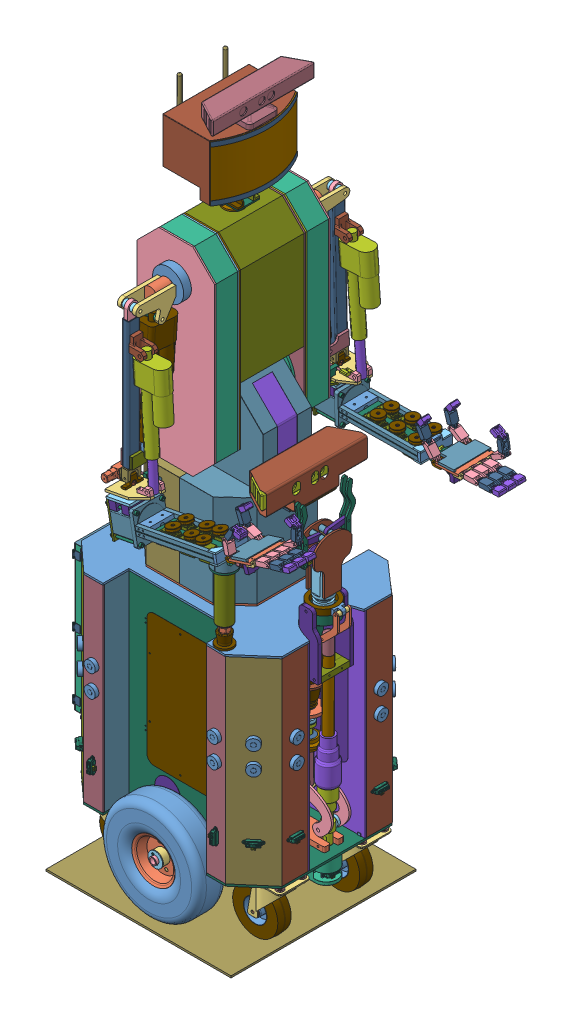
SolidWorks assembly sorbot, configuration По умолчанию. Lengths in mm. (continued)
Mates (geometry in assembly coordinates): (continued)
- Концентричный509: concentric anti-aligned: cylinder of HS-311 Hitec Standard Servo and Horn-9/HS-311-p2-1 through (220.6042 865.5775 -399.0607) axis (-0.012385 0.99968 0.022041) radius 4.064; cylinder of lower.arm.p9-11 through (220.5268 871.8255 -398.923) axis (0.012385 -0.99968 -0.022041) radius 12
- Совпадение938: coincident anti-aligned: plane of HS-311 Hitec Standard Servo and Horn-12/HS-311-p2-1 through (112.9596 871.5833 -448.3789) normal (-0.012385 0.99968 0.022041); plane of lower.arm.p9-8 through (110.7286 871.3708 -439.994) normal (0.012385 -0.99968 -0.022041)
- Совпадение939: coincident anti-aligned: plane of HS-311 Hitec Standard Servo and Horn-8/HS-311-p2-1 through (167.9775 872.3165 -450.7175) normal (-0.012385 0.99968 0.022041); plane of lower.arm.p9-10 through (165.7466 872.104 -442.3326) normal (0.012385 -0.99968 -0.022041)
- Совпадение940: coincident anti-aligned: plane of HS-311 Hitec Standard Servo and Horn-10/HS-311-p2-1 through (222.9951 873.0479 -452.9761) normal (-0.012385 0.99968 0.022041); plane of lower.arm.p9-12 through (220.7641 872.8354 -444.5912) normal (0.012385 -0.99968 -0.022041)
- Совпадение941: coincident anti-aligned: plane of HS-311 Hitec Standard Servo and Horn-9/HS-311-p2-1 through (222.7577 872.038 -407.3079) normal (-0.012385 0.99968 0.022041); plane of lower.arm.p9-11 through (220.5268 871.8255 -398.923) normal (0.012385 -0.99968 -0.022041)
- Совпадение942: coincident anti-aligned: plane of HS-311 Hitec Standard Servo and Horn-7/HS-311-p2-1 through (167.7668 871.4198 -410.168) normal (-0.012385 0.99968 0.022041); plane of lower.arm.p9-9 through (165.5359 871.2073 -401.783) normal (0.012385 -0.99968 -0.022041)
- Совпадение943: coincident anti-aligned: plane of HS-311 Hitec Standard Servo and Horn-11/HS-311-p2-1 through (112.7763 870.8034 -413.108) normal (-0.012385 0.99968 0.022041); plane of lower.arm.p9-7 through (110.5453 870.5909 -404.7231) normal (0.012385 -0.99968 -0.022041)
- Заблокировать452: lock: unknown of lower.arm.p8-3; unknown of palm.fixture.p4-6
- Заблокировать453: lock: unknown of lower.arm.p8-3; unknown of palm.fixture.p4-7
- Заблокировать454: lock: unknown of lower.arm.p8-3; unknown of palm.fixture.p4-8
- Заблокировать455: lock: unknown of lower.arm.p2-7; unknown of lower.arm.p8-3
- Заблокировать456: lock: unknown of lower.arm.p8-3; unknown of palm.fixture.p4-9
- Заблокировать458: lock: unknown of palm.fixture.p14-2; unknown of palm.p1-4
- Совпадение963: coincident anti-aligned: plane of palm.p1-4 through (362.2803 874.0257 -470.765) normal (-0.060104 0.997955 0.021755); plane of palm.p6-3 through (295.9379 868.6488 -407.401) normal (0.060104 -0.997955 -0.021755)
- Совпадение964: coincident anti-aligned: plane of palm.p1-4 through (362.2803 874.0257 -470.765) normal (-0.060104 0.997955 0.021755); plane of palm.p6-4 through (296.3955 869.3003 -436.0217) normal (0.060104 -0.997955 -0.021755)
- Совпадение965: coincident anti-aligned: plane of palm.p1-4 through (362.2803 874.0257 -470.765) normal (-0.060104 0.997955 0.021755); plane of palm.p5-3 through (330.0768 870.2924 -388.4794) normal (0.060104 -0.997955 -0.021755)
- Совпадение966: coincident anti-aligned: plane of palm.p1-4 through (362.2803 874.0257 -470.765) normal (-0.060104 0.997955 0.021755); plane of palm.p5-4 through (330.5285 871.7398 -453.6282) normal (0.060104 -0.997955 -0.021755)
- Заблокировать459: lock: unknown of palm.p1-4; unknown of palm.p6-3
- Заблокировать460: lock: unknown of palm.p1-4; unknown of palm.p6-4
- Заблокировать461: lock: unknown of palm.p1-4; unknown of palm.p5-3
- Заблокировать462: lock: unknown of palm.p1-4; unknown of palm.p5-4
- Совпадение967: coincident anti-aligned: plane of palm.p1-4 through (362.2803 874.0257 -470.765) normal (-0.060104 0.997955 0.021755); plane of palm.cap-2 through (306.1449 870.1321 -447.243) normal (0.060104 -0.997955 -0.021755)
- Совпадение968: coincident aligned: plane of palm.p1-4 through (286.8974 867.3169 -371.2793) normal (-0.998179 -0.059975 -0.006513); plane of palm.cap-2 through (286.6609 873.8329 -395.0363) normal (-0.998179 -0.059975 -0.006513)
- Совпадение969: coincident aligned: plane of palm.p1-4 through (286.8974 867.3169 -371.2793) normal (-0.005195 -0.022106 0.999742); plane of palm.cap-2 through (349.3088 877.0763 -370.7392) normal (-0.005195 -0.022106 0.999742)
- Заблокировать463: lock: unknown of palm.p1-4; unknown of palm.cap-2
- Совпадение970: coincident anti-aligned: plane of palm.p1-4 through (362.641 868.038 -470.8956) normal (0.060104 -0.997955 -0.021755); plane of palm.p3.m-3 through (319.6212 863.2737 -371.1987) normal (-0.060104 0.997955 0.021755)
- Совпадение971: coincident aligned: plane of palm.p1-4 through (286.8974 867.3169 -371.2793) normal (-0.005195 -0.022106 0.999742); plane of palm.p3.m-3 through (287.7592 869.3718 -371.2294) normal (-0.005195 -0.022106 0.999742)
- Совпадение972: coincident anti-aligned: plane of palm.p1-4 through (296.9 868.0051 -375.2131) normal (-0.998179 -0.059975 -0.006513); plane of palm.p3.m-3 through (296.6978 870.9282 -371.1485) normal (0.998179 0.059975 0.006513)
- Заблокировать464: lock: unknown of palm.p1-4; unknown of palm.p3.m-3
- Совпадение973: coincident anti-aligned: plane of palm.p1-4 through (362.641 868.038 -470.8956) normal (0.060104 -0.997955 -0.021755); plane of palm.p3.m-4 through (320.029 865.0091 -449.6784) normal (-0.060104 0.997955 0.021755)
- Совпадение974: coincident aligned: plane of palm.p1-4 through (287.4169 869.5276 -471.2535) normal (0.005195 0.022106 -0.999742); plane of palm.p3.m-4 through (288.2787 871.5825 -471.2036) normal (0.005195 0.022106 -0.999742)
- Совпадение975: coincident anti-aligned: plane of palm.p1-4 through (297.3779 870.0389 -467.1894) normal (-0.998179 -0.059975 -0.006513); plane of palm.p3.m-4 through (297.1057 872.6635 -449.6283) normal (0.998179 0.059975 0.006513)
- Заблокировать465: lock: unknown of palm.p1-4; unknown of palm.p3.m-4
- Совпадение976: coincident anti-aligned: plane of palm.p1-4 through (362.641 868.038 -470.8956) normal (0.060104 -0.997955 -0.021755); plane of palm.p3-2 through (343.5691 866.8921 -471.02) normal (-0.060104 0.997955 0.021755)
- Совпадение977: coincident aligned: plane of palm.p1-4 through (286.8974 867.3169 -371.2793) normal (-0.005195 -0.022106 0.999742); plane of palm.p3-2 through (370.5503 875.8487 -370.6559) normal (-0.005195 -0.022106 0.999742)
- Совпадение978: coincident anti-aligned: plane of palm.p1-4 through (361.7608 871.8151 -370.7908) normal (0.998179 0.059975 0.006513); plane of palm.p3-2 through (362.07 877.5186 -470.6889) normal (-0.998179 -0.059975 -0.006513)
- Заблокировать466: lock: unknown of palm.p1-4; unknown of palm.p3-2
- Концентричный510: concentric aligned: cylinder of palm.p3.m-3 through (292.5129 865.4279 -371.2919) axis (0.005195 0.022106 -0.999742) radius 1.5; cylinder of finger.p1-7 through (292.5155 865.439 -371.7918) axis (0.005195 0.022106 -0.999742) radius 1.5
- Совпадение979: coincident anti-aligned: plane of palm.p3.m-3 through (282.5498 857.4215 -389.0252) normal (-0.005195 -0.022106 0.999742); plane of finger.p1-7 through (295.546 853.9979 -389.0334) normal (0.005195 0.022106 -0.999742)
- Концентричный512: concentric aligned: cylinder of finger.p2-13 through (267.069 896.9455 -371.2273) axis (0.005195 0.022106 -0.999742) radius 1.5; cylinder of finger.p1-7 through (267.069 896.9455 -371.2273) axis (0.005195 0.022106 -0.999742) radius 1.5
- Совпадение980: coincident anti-aligned: plane of finger.p1-7 through (268.2587 888.6357 -387.9091) normal (-0.005195 -0.022106 0.999742); plane of finger.p2-13 through (268.1702 885.8361 -387.9715) normal (0.005195 0.022106 -0.999742)
- Концентричный513: concentric aligned: cylinder of finger.p2-13 through (248.7323 931.3594 -370.5616) axis (0.005195 0.022106 -0.999742) radius 1.5; cylinder of finger.p3-7 through (248.7328 931.3619 -370.6745) axis (0.005195 0.022106 -0.999742) radius 1.5
- Совпадение981: coincident anti-aligned: plane of finger.p2-13 through (248.3728 922.9913 -387.2528) normal (-0.005195 -0.022106 0.999742); plane of finger.p3-7 through (238.9673 925.751 -387.2406) normal (0.005195 0.022106 -0.999742)
- Заблокировать467: lock: unknown of palm.p3.m-3; unknown of finger.p1-7
- Заблокировать468: lock: unknown of finger.p1-7; unknown of finger.p2-13
- Заблокировать469: lock: unknown of finger.p2-13; unknown of finger.p3-7
- Концентричный514: concentric aligned: cylinder of palm.p3.m-4 through (292.9207 867.1633 -449.7716) axis (0.005195 0.022106 -0.999742) radius 1.5; cylinder of finger.p1-8 through (292.9233 867.1743 -450.2715) axis (0.005195 0.022106 -0.999742) radius 1.5
- Совпадение982: coincident anti-aligned: plane of palm.p3.m-4 through (282.9576 859.1568 -467.505) normal (-0.005195 -0.022106 0.999742); plane of finger.p1-8 through (299.5757 857.2919 -467.4599) normal (0.005195 0.022106 -0.999742)
- Концентричный515: concentric aligned: cylinder of finger.p1-8 through (258.7432 888.9029 -449.9687) axis (0.005195 0.022106 -0.999742) radius 1.5; cylinder of finger.p2-14 through (258.7432 888.9029 -449.9687) axis (0.005195 0.022106 -0.999742) radius 1.5
- Концентричный516: concentric aligned: cylinder of finger.p2-14 through (248.5939 926.551 -449.1889) axis (0.005195 0.022106 -0.999742) radius 1.5; cylinder of finger.p3-8 through (248.5934 926.5485 -449.0761) axis (0.005195 0.022106 -0.999742) radius 1.5
- Совпадение983: coincident anti-aligned: plane of finger.p2-14 through (246.2216 918.2291 -453.3863) normal (0.005195 0.022106 -0.999742); plane of finger.p3-8 through (238.7666 920.662 -453.3712) normal (-0.005195 -0.022106 0.999742)
- Совпадение984: coincident anti-aligned: plane of finger.p1-8 through (262.647 881.4001 -466.6185) normal (-0.005195 -0.022106 0.999742); plane of finger.p2-14 through (257.2443 877.8585 -466.7249) normal (0.005195 0.022106 -0.999742)
- Заблокировать470: lock: unknown of palm.p3.m-4; unknown of finger.p1-8
- Заблокировать471: lock: unknown of finger.p1-8; unknown of finger.p2-14
- Заблокировать472: lock: unknown of finger.p2-14; unknown of finger.p3-8
- Концентричный517: concentric: cylinder of palm.p3-2 through (337.7337 1179.9805 -460.0065) axis (-0.005196 -0.004798 0.999975) radius 1.5; cylinder of finger.p1-9 through (337.3284 1179.6063 -382.0084) axis (-0.005196 -0.004798 0.999975) radius 1.5
- Совпадение985: coincident: plane of palm.p3-2 through (336.9553 1167.4295 -365.0684) normal (0.005196 0.004798 -0.999975); plane of finger.p1-9 through (331.3626 1168.8569 -365.0906) normal (-0.005196 -0.004798 0.999975)
- Заблокировать473: lock: unknown of ?
- Концентричный518: concentric aligned: cylinder of finger.p1-9 through (406.8614 874.0028 -392.5138) axis (-0.005195 -0.022106 0.999742) radius 1.5; cylinder of finger.p2-15 through (406.8614 874.0028 -392.5138) axis (-0.005195 -0.022106 0.999742) radius 1.5
- Совпадение986: coincident anti-aligned: plane of finger.p1-9 through (399.5598 868.6975 -376.1648) normal (0.005195 0.022106 -0.999742); plane of finger.p2-15 through (396.4589 868.5111 -376.185) normal (-0.005195 -0.022106 0.999742)
- Заблокировать474: lock: unknown of finger.p1-9; unknown of finger.p2-15
- Концентричный519: concentric aligned: cylinder of finger.p2-15 through (445.7903 876.3419 -392.2597) axis (-0.005195 -0.022106 0.999742) radius 1.5; cylinder of finger.p3-9 through (445.7898 876.3394 -392.1469) axis (-0.005195 -0.022106 0.999742) radius 1.5
- Совпадение987: coincident anti-aligned: plane of finger.p2-15 through (438.4887 871.0365 -375.9107) normal (0.005195 0.022106 -0.999742); plane of finger.p3-9 through (435.3879 870.8502 -375.931) normal (-0.005195 -0.022106 0.999742)
- Заблокировать475: lock: unknown of finger.p2-15; unknown of finger.p3-9
- Концентричный520: concentric aligned: cylinder of palm.p3-2 through (366.8103 873.7971 -470.7465) axis (-0.005195 -0.022106 0.999742) radius 1.5; cylinder of finger.p1-10 through (366.5376 872.6365 -418.2601) axis (-0.005195 -0.022106 0.999742) radius 1.5
- Совпадение988: coincident anti-aligned: plane of palm.p3-2 through (371.5201 863.0505 -401.4418) normal (0.005195 0.022106 -0.999742); plane of finger.p1-10 through (355.6635 866.6048 -401.4456) normal (-0.005195 -0.022106 0.999742)
- Заблокировать476: lock: unknown of palm.p1-4; unknown of finger.p1-10
- Концентричный521: concentric aligned: cylinder of finger.p1-10 through (406.9938 874.5665 -418.0072) axis (-0.005195 -0.022106 0.999742) radius 1.5; cylinder of finger.p2-16 through (406.9938 874.5665 -418.0072) axis (-0.005195 -0.022106 0.999742) radius 1.5
- Совпадение989: coincident anti-aligned: plane of finger.p1-10 through (399.6923 869.2612 -401.6582) normal (0.005195 0.022106 -0.999742); plane of finger.p2-16 through (396.5914 869.0749 -401.6784) normal (-0.005195 -0.022106 0.999742)
- Заблокировать477: lock: unknown of finger.p1-10; unknown of finger.p2-16
- Концентричный522: concentric aligned: cylinder of finger.p2-16 through (445.9228 876.9056 -417.7532) axis (-0.005195 -0.022106 0.999742) radius 1.5; cylinder of finger.p3-10 through (445.9222 876.9031 -417.6403) axis (-0.005195 -0.022106 0.999742) radius 1.5
- Совпадение990: coincident anti-aligned: plane of finger.p2-16 through (438.6212 871.6002 -401.4042) normal (0.005195 0.022106 -0.999742); plane of finger.p3-10 through (435.5204 871.4139 -401.4244) normal (-0.005195 -0.022106 0.999742)
- Заблокировать478: lock: unknown of finger.p2-16; unknown of finger.p3-10
- Концентричный523: concentric aligned: cylinder of palm.p3-2 through (366.8103 873.7971 -470.7465) axis (-0.005195 -0.022106 0.999742) radius 1.5; cylinder of finger.p1-11 through (366.67 873.2002 -443.7535) axis (-0.005195 -0.022106 0.999742) radius 1.5
- Совпадение991: coincident anti-aligned: plane of palm.p3-2 through (371.6526 863.6142 -426.9352) normal (0.005195 0.022106 -0.999742); plane of finger.p1-11 through (355.7959 867.1685 -426.939) normal (-0.005195 -0.022106 0.999742)
- Заблокировать479: lock: unknown of palm.p3-2; unknown of finger.p1-11
- Концентричный524: concentric aligned: cylinder of finger.p1-11 through (407.1263 875.1303 -443.5006) axis (-0.005195 -0.022106 0.999742) radius 1.5; cylinder of finger.p2-17 through (407.1263 875.1303 -443.5006) axis (-0.005195 -0.022106 0.999742) radius 1.5
- Совпадение992: coincident anti-aligned: plane of finger.p1-11 through (399.8247 869.8249 -427.1516) normal (0.005195 0.022106 -0.999742); plane of finger.p2-17 through (396.7239 869.6386 -427.1718) normal (-0.005195 -0.022106 0.999742)
- Заблокировать480: lock: unknown of finger.p1-11; unknown of finger.p2-17
- Концентричный525: concentric aligned: cylinder of finger.p2-17 through (446.0553 877.4693 -443.2466) axis (-0.005195 -0.022106 0.999742) radius 1.5; cylinder of finger.p3-11 through (446.0547 877.4668 -443.1338) axis (-0.005195 -0.022106 0.999742) radius 1.5
- Совпадение993: coincident anti-aligned: plane of finger.p2-17 through (438.7537 872.1639 -426.8976) normal (0.005195 0.022106 -0.999742); plane of finger.p3-11 through (435.6528 871.9776 -426.9178) normal (-0.005195 -0.022106 0.999742)
- Заблокировать481: lock: unknown of finger.p2-17; unknown of finger.p3-11
- Концентричный526: concentric: cylinder of palm.p3-2 through (411.4236 915.5645 -460.8923) axis (-0.005196 -0.004798 0.999975) radius 1.5; cylinder of finger.p1-12 through (411.4158 915.5573 -459.3923) axis (-0.005196 -0.004798 0.999975) radius 1.5
- Совпадение994: coincident: plane of palm.p3-2 through (403.6967 906.0873 -442.4774) normal (0.005196 0.004798 -0.999975); plane of finger.p1-12 through (403.9419 905.7906 -442.4776) normal (-0.005196 -0.004798 0.999975)
- Концентричный527: concentric aligned: cylinder of finger.p1-12 through (401.144 895.2287 -468.5938) axis (-0.005195 -0.022106 0.999742) radius 1.5; cylinder of finger.p2-18 through (401.144 895.2287 -468.5938) axis (-0.005195 -0.022106 0.999742) radius 1.5
- Совпадение995: coincident anti-aligned: plane of finger.p1-12 through (397.1815 887.0261 -452.2916) normal (0.005195 0.022106 -0.999742); plane of finger.p2-18 through (407.0548 885.0276 -452.2844) normal (-0.005195 -0.022106 0.999742)
- Концентричный528: concentric aligned: cylinder of finger.p2-18 through (395.4647 933.8042 -467.7704) axis (-0.005195 -0.022106 0.999742) radius 1.5; cylinder of finger.p3-12 through (395.4641 933.8017 -467.6575) axis (-0.005195 -0.022106 0.999742) radius 1.5
- Совпадение996: coincident anti-aligned: plane of finger.p2-18 through (400.9231 926.6758 -451.3954) normal (0.005195 0.022106 -0.999742); plane of finger.p3-12 through (406.8279 932.1468 -451.2437) normal (-0.005195 -0.022106 0.999742)
- Заблокировать482: lock: unknown of palm.p3-2; unknown of finger.p1-12
- Заблокировать483: lock: unknown of finger.p1-12; unknown of finger.p2-18
- Заблокировать484: lock: unknown of finger.p2-18; unknown of finger.p3-12
- Заблокировать485: lock: unknown of arm.actuator100mm..p1-2; unknown of arm.actuator100mm.p2-2
- Концентричный529: concentric aligned: cylinder of body_axis-1 through (-20.0648 1016.5246 -50.7475) axis (0 0 -1) radius 9; cylinder of bodu.tilit.axis.enforcement-1 through (-20.0648 1016.5246 -50.7475) axis (0 0 -1) radius 9
- Совпадение999: coincident aligned: plane of body_axis-1 through (-20.0648 1016.5246 -221.0975) normal (0 0 -1); plane of bodu.tilit.axis.enforcement-1 through (-20.0648 1016.5246 -221.0975) normal (0 0 -1)
- Заблокировать486: lock: unknown of ?; unknown of arm.actuator.p2-4
- Заблокировать488: lock: unknown of turret.center-1; unknown of body_tilit_stud-1
- Заблокировать489: lock: unknown of turret.center-1; unknown of body_tilit_stud-9
- Заблокировать490: lock: unknown of turret.center-1; unknown of body_tilit_stud-8
- Заблокировать491: lock: unknown of turret.center-1; unknown of body_tilit_stud-7
- Заблокировать492: lock: unknown of turret.center-1; unknown of body_tilit_stud-6
- Заблокировать493: lock: unknown of turret.center-1; unknown of body_tilit_stud-5
- Совпадение1001: coincident anti-aligned: plane of m6.nut-1 through (8.0892 944.0246 -131.6914) normal (0 -1 0); plane of body_pivot_fixture-1 through (-20.0648 944.0246 -136.9555) normal (0 1 0)
- Концентричный530: concentric aligned: cylinder of body_tilit_stud-7 through (8.0892 955.7352 -137.4649) axis (0 -1 0) radius 3; cylinder of m6.nut-1 through (8.0892 949.5246 -137.4649) axis (0 -1 0) radius 3
- Совпадение1002: coincident anti-aligned: plane of m6.nut-2 through (-6.429 944.0246 -155.8188) normal (0 -1 0); plane of body_pivot_fixture-1 through (-20.0648 944.0246 -136.9555) normal (0 1 0)
- Концентричный531: concentric aligned: cylinder of body_tilit_stud-8 through (-6.429 955.7352 -161.5923) axis (0 -1 0) radius 3; cylinder of m6.nut-2 through (-6.429 949.5246 -161.5923) axis (0 -1 0) radius 3
- Совпадение1004: coincident anti-aligned: plane of m6.nut-3 through (-48.2188 944.0246 -130.6725) normal (0 -1 0); plane of body_pivot_fixture-1 through (-20.0648 944.0246 -136.9555) normal (0 1 0)
- Совпадение1005: coincident anti-aligned: plane of m6.nut-4 through (-34.583 944.0246 -155.3093) normal (0 -1 0); plane of body_pivot_fixture-1 through (-20.0648 944.0246 -136.9555) normal (0 1 0)
- Совпадение1006: coincident anti-aligned: plane of m6.nut-5 through (-5.5466 944.0246 -107.0546) normal (0 -1 0); plane of body_pivot_fixture-1 through (-20.0648 944.0246 -136.9555) normal (0 1 0)
- Совпадение1007: coincident anti-aligned: plane of m6.nut-6 through (-33.7006 944.0246 -106.5452) normal (0 -1 0); plane of body_pivot_fixture-1 through (-20.0648 944.0246 -136.9555) normal (0 1 0)
- Концентричный532: concentric aligned: cylinder of body_tilit_stud-1 through (-48.2188 955.7352 -136.446) axis (0 -1 0) radius 3; cylinder of m6.nut-3 through (-48.2188 949.5246 -136.446) axis (0 -1 0) radius 3
- Концентричный533: concentric aligned: cylinder of body_tilit_stud-9 through (-34.583 955.7352 -161.0828) axis (0 -1 0) radius 3; cylinder of m6.nut-4 through (-34.583 949.5246 -161.0828) axis (0 -1 0) radius 3
- Концентричный534: concentric aligned: cylinder of body_tilit_stud-6 through (-5.5466 955.7352 -112.8281) axis (0 -1 0) radius 3; cylinder of m6.nut-5 through (-5.5466 949.5246 -112.8281) axis (0 -1 0) radius 3
- Концентричный535: concentric aligned: cylinder of body_tilit_stud-5 through (-33.7006 955.7352 -112.3187) axis (0 -1 0) radius 3; cylinder of m6.nut-6 through (-33.7006 949.5246 -112.3187) axis (0 -1 0) radius 3
- Совпадение1008: coincident anti-aligned: plane of turret.center-1 through (-20.0648 662.7934 -136.9555) normal (0 -1 0); plane of m6.nut-12 through (-48.2188 662.7934 -130.6725) normal (0 1 0)
- Концентричный536: concentric aligned: cylinder of body_tilit_stud-1 through (-48.2188 955.7352 -136.446) axis (0 -1 0) radius 3; cylinder of m6.nut-12 through (-48.2188 662.7934 -136.446) axis (0 -1 0) radius 3
- Совпадение1009: coincident anti-aligned: plane of turret.center-1 through (-20.0648 662.7934 -136.9555) normal (0 -1 0); plane of m6.nut-11 through (-33.7006 662.7934 -106.5452) normal (0 1 0)
- Концентричный537: concentric aligned: cylinder of body_tilit_stud-5 through (-33.7006 955.7352 -112.3187) axis (0 -1 0) radius 3; cylinder of m6.nut-11 through (-33.7006 662.7934 -112.3187) axis (0 -1 0) radius 3
- Совпадение1010: coincident anti-aligned: plane of turret.center-1 through (-20.0648 662.7934 -136.9555) normal (0 -1 0); plane of m6.nut-7 through (-5.5466 662.7934 -107.0546) normal (0 1 0)
- Концентричный538: concentric aligned: cylinder of body_tilit_stud-6 through (-5.5466 955.7352 -112.8281) axis (0 -1 0) radius 3; cylinder of m6.nut-7 through (-5.5466 662.7934 -112.8281) axis (0 -1 0) radius 3
- Совпадение1011: coincident anti-aligned: plane of turret.center-1 through (-20.0648 662.7934 -136.9555) normal (0 -1 0); plane of m6.nut-8 through (-34.583 662.7934 -155.3093) normal (0 1 0)
- Концентричный539: concentric aligned: cylinder of body_tilit_stud-9 through (-34.583 955.7352 -161.0828) axis (0 -1 0) radius 3; cylinder of m6.nut-8 through (-34.583 662.7934 -161.0828) axis (0 -1 0) radius 3
- Совпадение1012: coincident anti-aligned: plane of turret.center-1 through (-20.0648 662.7934 -136.9555) normal (0 -1 0); plane of m6.nut-10 through (-6.429 662.7934 -155.8188) normal (0 1 0)
- Концентричный540: concentric aligned: cylinder of body_tilit_stud-8 through (-6.429 955.7352 -161.5923) axis (0 -1 0) radius 3; cylinder of m6.nut-10 through (-6.429 662.7934 -161.5923) axis (0 -1 0) radius 3
- Совпадение1013: coincident anti-aligned: plane of turret.center-1 through (-20.0648 662.7934 -136.9555) normal (0 -1 0); plane of m6.nut-9 through (8.0892 662.7934 -131.6914) normal (0 1 0)
- Концентричный541: concentric aligned: cylinder of body_tilit_stud-7 through (8.0892 955.7352 -137.4649) axis (0 -1 0) radius 3; cylinder of m6.nut-9 through (8.0892 662.7934 -137.4649) axis (0 -1 0) radius 3
- Концентричный542: concentric anti-aligned: cylinder of body_tilt_lever_axis-1 through (-99.3474 976.856 -80.4875) axis (0 0 -1) radius 5; cylinder of body.tilt.intermediate.enforce-1 through (-99.3474 976.856 -149.5942) axis (0 0 1) radius 5
- Совпадение1014: coincident anti-aligned: plane of body_tilt_lever-2 through (-97.2168 978.7734 -124.5942) normal (0 0 -1); plane of body.tilt.intermediate.enforce-1 through (-99.3474 976.856 -124.5942) normal (0 0 1)
- Заблокировать498: lock: unknown of arm.fixture.cap-2; unknown of body.frame.p1-left-1
- Заблокировать499: lock: unknown of body.tilit.enforcement-2; unknown of body.frame.p1-left-1
- Заблокировать500: lock: unknown of body.frame.p2-1; unknown of body.frame.p1-left-1
- Совпадение1021: coincident anti-aligned: plane of body.frame.p1-left-1 through (92.5148 1436.2936 -222.3595) normal (0 0 1); plane of arm.drive.motor.pair-1 through (3.7745 1243.7974 -222.3595) normal (0 0 -1)
- Совпадение1022: coincident anti-aligned: plane of body.frame.p1-3 through (92.5097 1436.2936 -50.7442) normal (0 0 -1); plane of arm.drive.motor-1 through (-20.8275 1162.0905 -50.7442) normal (0 0 1)
- Концентричный547: concentric anti-aligned: cylinder of arm.actuator.p2-5 through (-12.3063 966.5653 -383.5224) axis (-0.000486 0.995617 0.093518) radius 10; cylinder of arm.actuator-5/arm.actuator.p1-1 through (-12.3974 1153.2752 -365.9848) axis (0.000486 -0.995617 -0.093518) radius 10
- Концентричный549: concentric anti-aligned: cylinder of arm.drive.p3-1 through (3.7745 1243.7974 -65.7442) axis (0 0 1) radius 6; cylinder of arm.drive.p5-1 through (3.7745 1243.7974 -50.7442) axis (0 0 -1) radius 6
- Совпадение1023: coincident anti-aligned: plane of body.frame.p1-3 through (92.5097 1436.2936 -50.7442) normal (0 0 -1); plane of arm.drive.p5-1 through (3.7745 1243.7974 -50.7442) normal (0 0 1)
- Концентричный550: concentric anti-aligned: cylinder of arm.drive.p3-1 through (3.7745 1243.7974 -65.7442) axis (0 0 1) radius 6; cylinder of arm.drive.p6-1 through (3.7745 1243.7974 -50.7442) axis (0 0 -1) radius 7
- Совпадение1024: coincident anti-aligned: plane of body.frame.p1-3 through (92.5097 1436.2936 -50.7442) normal (0 0 -1); plane of arm.drive.p6-1 through (3.7745 1243.7974 -50.7442) normal (0 0 1)
- Концентричный551: concentric anti-aligned: cylinder of arm.drive.p3-1 through (3.7745 1243.7974 -65.7442) axis (0 0 1) radius 6; cylinder of arm.drive.motor.pair-1 through (3.7745 1243.7974 -192.8595) axis (0 0 -1) radius 8
- Заблокировать504: lock: unknown of body.frame.p1-left-1; unknown of arm.drive.motor.pair-1
- Совпадение1028: coincident anti-aligned: plane of body.frame.p1-left-1 through (92.5148 1436.2936 -222.3595) normal (0 0 1); plane of arm.drive.p3-2 through (-20.8275 1162.0905 -222.3595) normal (0 0 -1)
- Концентричный553: concentric anti-aligned: cylinder of arm.drive.motor-1 through (-20.8275 1162.0905 -80.2442) axis (0 0 1) radius 8; cylinder of arm.drive.p3-2 through (-20.8275 1162.0905 -207.3595) axis (0 0 -1) radius 6
- Концентричный554: concentric anti-aligned: cylinder of arm.drive.p3-2 through (-20.8275 1162.0905 -207.3595) axis (0 0 -1) radius 6; cylinder of arm.drive.p5-2 through (-20.8275 1162.0905 -222.3595) axis (0 0 1) radius 6
- Совпадение1029: coincident anti-aligned: plane of body.frame.p1-left-1 through (92.5148 1436.2936 -222.3595) normal (0 0 1); plane of arm.drive.p5-2 through (-20.8275 1162.0905 -222.3595) normal (0 0 -1)
- Совпадение1030: coincident anti-aligned: plane of body.frame.p1-left-1 through (92.5148 1436.2936 -222.3595) normal (0 0 1); plane of arm.drive.p6-2 through (-20.8275 1162.0905 -222.3595) normal (0 0 -1)
- Концентричный555: concentric anti-aligned: cylinder of arm.drive.p3-2 through (-20.8275 1162.0905 -207.3595) axis (0 0 -1) radius 6; cylinder of arm.drive.p6-2 through (-20.8275 1162.0905 -222.3595) axis (0 0 1) radius 7
- Заблокировать505: lock: unknown of body.frame.p1-3; unknown of arm.drive.motor-1
- Заблокировать506: lock: unknown of body.frame.p1-left-1; unknown of arm.drive.p6-2
- Заблокировать507: lock: unknown of body.frame.p1-3; unknown of arm.drive.p6-1
- Заблокировать508: lock: unknown of body.frame.p1-3; unknown of arm.drive.p6-1
- Заблокировать510: lock: unknown of ?; unknown of arm.actuator.p2-5
- Концентричный559: concentric anti-aligned: cylinder of arm.drive.p3-2 through (-20.8275 1162.0905 -207.3595) axis (0 0 -1) radius 6; cylinder of m14.nut-1 through (-20.8275 1162.0905 -128.9852) axis (0 0 1) radius 7
- Совпадение1034: coincident anti-aligned: plane of arm.drive.p7-2 through (-42.4721 1162.0905 -109.4852) normal (0 1 0); plane of arm.drive.p7-3 through (-42.4721 1162.0905 -137.4852) normal (0 -1 0)
- Совпадение1035: coincident aligned: plane of arm.drive.p7-2 through (12.3724 1162.0905 -109.4852) normal (0 0 1); plane of arm.drive.p7-3 through (12.3724 1162.0905 -109.4852) normal (0 0 1)
- Совпадение1036: coincident aligned: plane of arm.drive.p7-2 through (-42.4721 1162.0905 -137.4852) normal (-1 0 0); plane of arm.drive.p7-3 through (-42.4721 1162.0905 -109.4852) normal (-1 0 0)
- Концентричный560: concentric anti-aligned: cylinder of arm.drive.p2-pair-1 through (10.8018 1164.5905 -123.4852) axis (0 -1 0) radius 2.5; cylinder of arm.drive.p7-3 through (10.8018 1162.0905 -123.4852) axis (0 1 0) radius 2.5
- Совпадение1038: coincident anti-aligned: plane of m14.nut-1 through (-8.1258 1162.0905 -128.9852) normal (0 0 -1); plane of arm.drive.p7-3 through (-33.7738 1162.0905 -128.9852) normal (0 0 1)
- Заблокировать511: lock: unknown of m14.nut-1; unknown of arm.drive.p7-3
- Совпадение1040: coincident anti-aligned: plane of arm.drive.p7-4 through (-9.0342 1232.7974 -150.3) normal (0 1 0); plane of m14.nut-2 through (-2.5764 1232.7974 -139.8) normal (0 -1 0)
- Совпадение1041: coincident anti-aligned: plane of m14.nut-2 through (-2.5764 1254.7974 -150.3) normal (0 0 -1); plane of arm.drive.p7-4 through (-9.0341 1243.9206 -150.3) normal (0 0 1)
- Совпадение1042: coincident: plane of arm.drive.p7-4 through (16.4762 1232.7974 -150.3) normal (-1 0 0); line of m14.nut-2 through (16.4762 1243.7974 -140.8) axis (0 0 -1)
- Заблокировать512: lock: unknown of arm.drive.p7-4; unknown of m14.nut-2
- Концентричный562: concentric anti-aligned: cylinder of m14.nut-2 through (3.7745 1243.7974 -139.8) axis (0 0 -1) radius 7; cylinder of arm.drive.p3-1 through (3.7745 1243.7974 -65.7442) axis (0 0 1) radius 6
- Совпадение1043: coincident anti-aligned: plane of arm.drive.p7-5 through (-17.7325 1243.9206 -159.3) normal (0 -1 0); plane of arm.drive.p7-4 through (-17.7325 1243.9206 -131.3) normal (0 1 0)
- Концентричный563: concentric anti-aligned: cylinder of arm.drive.p7-4 through (35.5414 1243.9206 -145.3) axis (0 -1 0) radius 2.5; cylinder of arm.drive.p7-5 through (35.5414 1243.9206 -145.3) axis (0 1 0) radius 2.5
- Совпадение1045: coincident aligned: plane of arm.drive.p7-4 through (-17.7325 1243.9206 -159.3) normal (-1 0 0); plane of arm.drive.p7-5 through (-17.7325 1243.9206 -131.3) normal (-1 0 0)
- Совпадение1046: coincident aligned: plane of arm.drive.p7-4 through (37.112 1243.9206 -131.3) normal (0 0 1); plane of arm.drive.p7-5 through (37.112 1243.9206 -131.3) normal (0 0 1)
- Концентричный564: concentric anti-aligned: cylinder of arm.drive.p2-1 through (35.5414 1246.2974 -145.3) axis (0 -1 0) radius 2.5; cylinder of arm.drive.p7-5 through (35.5414 1243.9206 -145.3) axis (0 1 0) radius 2.5
- Совпадение1047: coincident anti-aligned: plane of body.frame.p4-4 through (-117.3772 1436.2936 -230.3595) normal (0 0 -1); plane of arm.drive.p1.m1-1 through (28.6519 1174.5905 -230.3595) normal (0 0 1)
- Совпадение1048: coincident anti-aligned: plane of body.frame.p4-4 through (-117.3772 1436.2936 -230.3595) normal (0 0 -1); plane of arm.drive.p1.m1-2 through (28.6519 1159.5905 -230.3595) normal (0 0 1)
- Параллельность203: parallel anti-aligned: plane of arm.drive.p1.m1-1 through (28.6519 1164.5905 -234.3595) normal (0 -1 0); plane of arm.drive.p1.m1-2 through (28.6519 1159.5905 -234.3595) normal (0 1 0)
- Совпадение1051: coincident anti-aligned: plane of arm.drive.p2-pair-1 through (48.6519 1164.5905 -237.3595) normal (0 1 0); plane of arm.drive.p1.m1-1 through (28.6519 1164.5905 -234.3595) normal (0 -1 0)
- Совпадение1052: coincident aligned: plane of arm.drive.p1.m1-1 through (68.6519 1174.5904 -230.3595) normal (1 0 0); plane of arm.drive.p1.m1-2 through (68.6519 1159.5904 -230.3595) normal (1 0 0)
- Совпадение1053: coincident anti-aligned: plane of arm.drive.p2-pair-1 through (48.6519 1159.5905 -237.3595) normal (0 -1 0); plane of arm.drive.p1.m1-2 through (28.6519 1159.5905 -234.3595) normal (0 1 0)
- Заблокировать513: lock: unknown of body.frame.p4-4; unknown of arm.drive.p1.m1-1
- Заблокировать514: lock: unknown of body.frame.p4-4; unknown of arm.drive.p1.m1-2
- Концентричный565: concentric aligned: cylinder of arm.drive.p2-pair-1 through (48.6519 1164.5905 -237.3595) axis (0 -1 0) radius 2.5; cylinder of arm.drive.p1.m1-2 through (48.6519 1159.5905 -237.3595) axis (0 -1 0) radius 2.5
- Концентричный566: concentric anti-aligned: cylinder of shoulder.bearing.housing-3 through (-12.6499 1335.3853 -313.3595) axis (0 0 1) radius 15.5; cylinder of body.frame.p4.external-1 through (-12.6499 1335.3853 -288.3595) axis (0 0 -1) radius 21
- Заблокировать516: lock: unknown of body.frame.p5-2; unknown of body.frame.p4.external-1
- Заблокировать517: lock: unknown of shoulder.bearing.housing-3; unknown of body.frame.p4.external-1
- Заблокировать518: lock: unknown of arm.lift.actuator.fixture.p3-4; unknown of body.frame.p4.external-1
- Концентричный567: concentric aligned: cylinder of shoulder.bearing.housing-1 through (-12.7629 1335.3853 40.2558) axis (0 0 -1) radius 15.5; cylinder of body.frame.p4.external-2 through (-12.7629 1335.3853 19.2558) axis (0 0 -1) radius 21
- Заблокировать520: lock: unknown of body.frame.p5-1; unknown of body.frame.p4.external-2
- Заблокировать522: lock: unknown of arm.lift.actuator.fixture.p3-1; unknown of body.frame.p4.external-2
- Заблокировать523: lock: unknown of shoulder.bearing.housing-1; unknown of body.frame.p4.external-2
- Заблокировать524: lock: unknown of arm.lift.actuator.fixture.p2-1; unknown of arm.lift.actuator.fixture.p3-1
- Совпадение1061: coincident anti-aligned: plane of arm.drive.p2-1 through (45.4163 1246.2974 -35.7442) normal (0 1 0); plane of arm.drive.p1.m1-4 through (65.4163 1246.2974 -38.7442) normal (0 -1 0)
- Совпадение1064: coincident aligned: plane of arm.drive.p1.m1-3 through (65.4163 1241.2974 -42.7442) normal (1 0 0); plane of arm.drive.p1.m1-4 through (65.4163 1256.2974 -42.7442) normal (1 0 0)
- Совпадение1065: coincident anti-aligned: plane of arm.drive.p2-1 through (45.4163 1241.2974 -35.7442) normal (0 -1 0); plane of arm.drive.p1.m1-3 through (65.4163 1241.2974 -38.7442) normal (0 1 0)
- Концентричный568: concentric aligned: cylinder of arm.drive.p2-1 through (45.4163 1246.2974 -35.7442) axis (0 -1 0) radius 2.5; cylinder of arm.drive.p1.m1-4 through (45.4163 1256.2974 -35.7442) axis (0 -1 0) radius 2.5
- Концентричный569: concentric anti-aligned: cylinder of shoulder.bearing.housing-2 through (-12.4903 1335.516 -67.7442) axis (0 0 1) radius 15.5; cylinder of body.frame.p4.right-1 through (-12.4903 1335.516 -42.7442) axis (0 0 -1) radius 12.5
- Заблокировать527: lock: unknown of arm.lift.actuator.fixture.p3-2; unknown of body.frame.p4.right-1
- Заблокировать528: lock: unknown of shoulder.bearing.housing-2; unknown of body.frame.p4.right-1
- Заблокировать529: lock: unknown of body.frame.p5-1; unknown of body.frame.p4.right-1
- Заблокировать530: lock: unknown of arm.drive.p1.m1-4; unknown of body.frame.p4.right-1
- Заблокировать531: lock: unknown of arm.drive.p1.m1-3; unknown of body.frame.p4.right-1
- Совпадение1067: coincident anti-aligned: plane of body.frame.p1-3 through (92.5097 1436.2936 -46.7442) normal (0 0 1); plane of body.frame.p4.right-1 through (-117.4903 1436.2936 -46.7442) normal (0 0 -1)
- Совпадение1026: coincident anti-aligned: plane of body.frame.p4-4 through (-117.3772 1436.2936 -226.3595) normal (0 0 1); plane of body.frame.p1-left-1 through (92.5148 1436.2936 -226.3595) normal (0 0 -1)
- Концентричный570: concentric aligned: cylinder of arm.drive.motor-1 through (-20.8275 1162.0905 -80.2442) axis (0 0 1) radius 8; cylinder of arm.drive.p8-1 through (-20.8275 1162.0905 -80.2442) axis (0 0 1) radius 8
- Совпадение1069: coincident anti-aligned: plane of arm.drive.motor-1 through (-20.8275 1162.0905 -72.7442) normal (0 0 -1); plane of arm.drive.p8-1 through (-20.8275 1162.0905 -72.7442) normal (0 0 1)
- Концентричный571: concentric aligned: cylinder of arm.drive.motor.pair-1 through (3.7745 1243.7974 -192.8595) axis (0 0 -1) radius 8; cylinder of arm.drive.p8-2 through (3.7745 1243.7974 -192.8595) axis (0 0 -1) radius 8
- Совпадение1070: coincident anti-aligned: plane of arm.drive.motor.pair-1 through (3.7745 1243.7974 -200.3595) normal (0 0 1); plane of arm.drive.p8-2 through (3.7745 1243.7974 -200.3595) normal (0 0 -1)
- Концентричный572: concentric aligned: cylinder of man1.drive1-1 through (-119.3768 773.978 -141.6211) axis (0 -1 0) radius 6; cylinder of tilt.thread.rod.fixture.2-1 through (-119.3768 819.5591 -141.6211) axis (0 -1 0) radius 12
- Совпадение1071: coincident anti-aligned: plane of turret.table-1 through (-20.0648 612.7934 -360.2969) normal (0 1 0); plane of body.tilit.planetary.drive.fixture.p1-1 through (-119.3768 612.7934 -141.6211) normal (0 -1 0)
- Концентричный573: concentric aligned: cylinder of man1.drive1-1 through (-119.3768 703.728 -141.6211) axis (0 -1 0) radius 19; cylinder of body.tilit.planetary.drive.fixture.p1-1 through (-119.3768 622.7934 -141.6211) axis (0 -1 0) radius 42.5
- Заблокировать532: lock: unknown of turret.table-1; unknown of body.tilit.planetary.drive.fixture.p1-1
- Совпадение1072: coincident anti-aligned: plane of body.tilit.planetary.drive.fixture.p1-1 through (-119.3768 622.7934 -141.6211) normal (0 1 0); plane of body.tilit.planetary.drive.fixture.p2-1 through (-119.3768 622.7934 -141.6211) normal (0 -1 0)
- Концентричный575: concentric aligned: cylinder of body.tilit.planetary.drive.fixture.p1-1 through (-119.3768 622.7934 -141.6211) axis (0 -1 0) radius 42.5; cylinder of body.tilit.planetary.drive.fixture.p2-1 through (-119.3768 626.7934 -141.6211) axis (0 -1 0) radius 42.5
- Концентричный577: concentric aligned: cylinder of man1.drive1-1 through (-119.3768 773.978 -141.6211) axis (0 -1 0) radius 6; cylinder of tilt.thread.rod.fixture.2-2 through (-119.3768 792.5591 -141.6211) axis (0 -1 0) radius 8
- Совпадение1073: coincident anti-aligned: plane of tilt.thread.rod.fixture.2-1 through (-119.3768 793.5591 -141.6211) normal (0 -1 0); plane of tilt.thread.rod.fixture.2-2 through (-119.3768 793.5591 -141.6211) normal (0 1 0)
- Концентричный578: concentric aligned: cylinder of man1.drive1-1 through (-119.3768 703.728 -141.6211) axis (0 -1 0) radius 19; cylinder of body.tilit.planetary.drive.fixture.p3-1 through (-119.3768 703.728 -141.6211) axis (0 -1 0) radius 19
- Совпадение1074: coincident anti-aligned: plane of man1.drive1-1 through (-119.3768 703.728 -141.6211) normal (0 -1 0); plane of body.tilit.planetary.drive.fixture.p3-1 through (-119.3768 703.728 -141.6211) normal (0 1 0)
- Концентричный579: concentric aligned: cylinder of man1.drive1-1 through (-119.3768 761.728 -141.6211) axis (0 -1 0) radius 14.75; cylinder of body.tilit.planetary.drive.fixture.p4-1 through (-119.3768 762.9526 -141.6211) axis (0 -1 0) radius 14.8
- Заблокировать533: lock: unknown of man1.drive1-1; unknown of body.tilit.planetary.drive.fixture.p4-1
- Концентричный580: concentric anti-aligned: cylinder of body.tilit.planetary.drive.fixture.p3-1 through (-148.8664 695.728 -141.6211) axis (0 1 0) radius 2.5; cylinder of body.tilit.planetary.drive.fixture.p5-1 through (-148.8664 769.7934 -141.6211) axis (0 -1 0) radius 2.5
- Совпадение1076: coincident aligned: plane of body.tilit.planetary.drive.fixture.p1-1 through (-119.3768 612.7934 -141.6211) normal (0 -1 0); plane of body.tilit.planetary.drive.fixture.p5-1 through (-148.8664 612.7934 -141.6211) normal (0 -1 0)
- Совпадение1077: coincident anti-aligned: plane of body.tilit.planetary.drive.fixture.p1-1 through (-148.8664 618.7934 -141.6211) normal (0 -1 0); plane of m6.nut-13 through (-148.8664 618.7934 -135.8476) normal (0 1 0)
- Концентричный581: concentric aligned: cylinder of body.tilit.planetary.drive.fixture.p5-1 through (-148.8664 769.7934 -141.6211) axis (0 -1 0) radius 2.5; cylinder of m6.nut-13 through (-148.8664 618.7934 -141.6211) axis (0 -1 0) radius 3
- Концентричный582: concentric aligned: cylinder of body.tilit.planetary.drive.fixture.p1-1 through (-119.3768 624.7934 -112.1315) axis (0 -1 0) radius 2.5; cylinder of body.tilit.planetary.drive.fixture.p5-3 through (-119.3768 769.7934 -112.1315) axis (0 -1 0) radius 2.5
- Концентричный583: concentric aligned: cylinder of body.tilit.planetary.drive.fixture.p1-1 through (-89.8872 624.7934 -141.6211) axis (0 -1 0) radius 2.5; cylinder of body.tilit.planetary.drive.fixture.p5-2 through (-89.8872 769.7934 -141.6211) axis (0 -1 0) radius 2.5
- Концентричный584: concentric aligned: cylinder of body.tilit.planetary.drive.fixture.p1-1 through (-119.3768 624.7934 -171.1107) axis (0 -1 0) radius 2.5; cylinder of body.tilit.planetary.drive.fixture.p5-4 through (-119.3768 769.7934 -171.1107) axis (0 -1 0) radius 2.5
- Совпадение1078: coincident aligned: plane of body.tilit.planetary.drive.fixture.p1-1 through (-119.3768 612.7934 -141.6211) normal (0 -1 0); plane of body.tilit.planetary.drive.fixture.p5-4 through (-119.3768 612.7934 -171.1107) normal (0 -1 0)
- Совпадение1079: coincident aligned: plane of body.tilit.planetary.drive.fixture.p1-1 through (-119.3768 612.7934 -141.6211) normal (0 -1 0); plane of body.tilit.planetary.drive.fixture.p5-3 through (-119.3768 612.7934 -112.1315) normal (0 -1 0)
- Совпадение1080: coincident aligned: plane of body.tilit.planetary.drive.fixture.p1-1 through (-119.3768 612.7934 -141.6211) normal (0 -1 0); plane of body.tilit.planetary.drive.fixture.p5-2 through (-89.8872 612.7934 -141.6211) normal (0 -1 0)
- Концентричный585: concentric aligned: cylinder of body.tilit.planetary.drive.fixture.p5-4 through (-119.3768 769.7934 -171.1107) axis (0 -1 0) radius 2.5; cylinder of m6.nut-15 through (-119.3768 618.7934 -171.1107) axis (0 -1 0) radius 3
- Концентричный586: concentric aligned: cylinder of body.tilit.planetary.drive.fixture.p5-2 through (-89.8872 769.7934 -141.6211) axis (0 -1 0) radius 2.5; cylinder of m6.nut-14 through (-89.8872 618.7934 -141.6211) axis (0 -1 0) radius 3
- Концентричный587: concentric aligned: cylinder of body.tilit.planetary.drive.fixture.p5-3 through (-119.3768 769.7934 -112.1315) axis (0 -1 0) radius 2.5; cylinder of m6.nut-16 through (-119.3768 618.7934 -112.1315) axis (0 -1 0) radius 3
- Совпадение1081: coincident anti-aligned: plane of body.tilit.planetary.drive.fixture.p1-1 through (-119.3768 618.7934 -112.1315) normal (0 -1 0); plane of m6.nut-16 through (-113.8446 618.7934 -113.783) normal (0 1 0)
- Совпадение1082: coincident anti-aligned: plane of body.tilit.planetary.drive.fixture.p1-1 through (-89.8872 618.7934 -141.6211) normal (0 -1 0); plane of m6.nut-14 through (-89.8872 618.7934 -135.8476) normal (0 1 0)
- Совпадение1083: coincident anti-aligned: plane of body.tilit.planetary.drive.fixture.p1-1 through (-119.3768 618.7934 -171.1107) normal (0 -1 0); plane of m6.nut-15 through (-114.7531 618.7934 -167.6531) normal (0 1 0)
- Совпадение1084: coincident anti-aligned: plane of body.tilit.planetary.drive.fixture.p4-1 through (-119.3768 762.9526 -141.6211) normal (0 1 0); plane of m6.nut-17 through (-122.5346 762.9526 -107.2981) normal (0 -1 0)
- Совпадение1085: coincident anti-aligned: plane of body.tilit.planetary.drive.fixture.p4-1 through (-119.3768 762.9526 -141.6211) normal (0 1 0); plane of m6.nut-18 through (-93.045 762.9526 -136.7877) normal (0 -1 0)
- Совпадение1086: coincident anti-aligned: plane of m6.nut-19 through (-122.5346 762.9526 -166.2773) normal (0 -1 0); plane of body.tilit.planetary.drive.fixture.p4-1 through (-119.3768 762.9526 -141.6211) normal (0 1 0)
- Совпадение1087: coincident anti-aligned: plane of body.tilit.planetary.drive.fixture.p4-1 through (-119.3768 762.9526 -141.6211) normal (0 1 0); plane of m6.nut-20 through (-152.0242 762.9526 -136.7877) normal (0 -1 0)
- Концентричный588: concentric anti-aligned: cylinder of body.tilit.planetary.drive.fixture.p5-1 through (-148.8664 769.7934 -141.6211) axis (0 -1 0) radius 2.5; cylinder of m6.nut-20 through (-148.8664 762.9526 -141.6211) axis (0 1 0) radius 3
- Концентричный589: concentric anti-aligned: cylinder of body.tilit.planetary.drive.fixture.p5-4 through (-119.3768 769.7934 -171.1107) axis (0 -1 0) radius 2.5; cylinder of m6.nut-19 through (-119.3768 762.9526 -171.1107) axis (0 1 0) radius 3
- Концентричный590: concentric anti-aligned: cylinder of body.tilit.planetary.drive.fixture.p5-2 through (-89.8872 769.7934 -141.6211) axis (0 -1 0) radius 2.5; cylinder of m6.nut-18 through (-89.8872 762.9526 -141.6211) axis (0 1 0) radius 3
- Концентричный591: concentric anti-aligned: cylinder of body.tilit.planetary.drive.fixture.p5-3 through (-119.3768 769.7934 -112.1315) axis (0 -1 0) radius 2.5; cylinder of m6.nut-17 through (-119.3768 762.9526 -112.1315) axis (0 1 0) radius 3
- Касательный36: tangent anti-aligned: cylinder of shoulder.p6-2 through (-12.6483 1335.4904 4.6679) axis (0 0 1) radius 19.94; plane of m6.nut-21 through (-29.5996 1324.99 15.6749) normal (0.850111 0.526603 0)
- Концентричный592: concentric aligned: cylinder of shoulder.p6-2 through (-72.9636 1298.128 9.9014) axis (0.850111 0.526603 0) radius 3; cylinder of m6.nut-21 through (-34.2752 1322.0936 9.9014) axis (0.850111 0.526603 0) radius 3
- Концентричный593: concentric aligned: cylinder of m6.6.50mm-1 through (-38.2027 1319.6607 9.9014) axis (0.850111 0.526603 0) radius 3; cylinder of shoulder.p6-2 through (-72.9636 1298.128 9.9014) axis (0.850111 0.526603 0) radius 3
- Касательный37: tangent anti-aligned: cylinder of shoulder.p6-2 through (-12.6483 1335.4904 4.6679) axis (0 0 1) radius 19.94; plane of m6.6.50mm-1 through (4.3029 1345.9909 9.9014) normal (-0.850111 -0.526603 0)
- Концентричный594: concentric anti-aligned: cylinder of shoulder.p6-2 through (-35.3987 1340.8364 -1.3321) axis (0 0 1) radius 2; cylinder of m4.nut-1 through (-35.3987 1340.8364 9.6679) axis (0 0 -1) radius 2
- Совпадение1088: coincident anti-aligned: plane of shoulder.p6-2 through (-12.6483 1335.4904 4.6679) normal (0 0 1); plane of m4.nut-1 through (-35.3987 1336.8758 4.6679) normal (0 0 -1)
- Концентричный595: concentric anti-aligned: cylinder of shoulder.p4-2 through (-12.6483 1335.4904 0.2558) axis (0 0 -1) radius 15; cylinder of shoulder.p6-2 through (-12.6483 1335.4904 -1.3321) axis (0 0 1) radius 15
- Совпадение1089: coincident anti-aligned: plane of arm.lift.actuator.fixture.p3-2 through (-88.5767 993.1387 -35.7442) normal (0 0 1); plane of m4.nut-2 through (-103.2224 993.9386 -35.7442) normal (0 0 -1)
- Концентричный596: concentric anti-aligned: cylinder of arm.lift.actuator.fixture.p3-2 through (-103.2224 997.8992 -42.7442) axis (0 0 1) radius 2; cylinder of m4.nut-2 through (-103.2224 997.8992 -30.7442) axis (0 0 -1) radius 2
- Заблокировать534: lock: unknown of lower.arm.p2-2; unknown of lower.arm.p3-1
- Заблокировать535: lock: unknown of lower.arm.p2-4; unknown of lower.arm.p3-1
- Концентричный598: concentric aligned: cylinder of forearm.rotate.p9-1 through (-12.6985 939.7014 123.1926) axis (0 0 1) radius 2.5; cylinder of arm.rotate.p8-1 through (-12.6985 939.7014 130.5417) axis (0 0 1) radius 2.5
- Совпадение1090: coincident: plane of forearm.rotate.p9-1 through (-2.9289 953.7014 150.5417) normal (0 0 -1); plane of arm.rotate.p8-1 through (-12.4887 947.5088 150.5417) normal (0 0 1)
- Параллельность206: parallel aligned: plane of arm.p1.m-1 through (-18.263 964.7884 156.4102) normal (0 0 1); plane of body.frame.p4.external-2 through (-117.7515 1436.1748 19.2558) normal (0 0 1)
- Совпадение1094: coincident aligned: plane of lower.arm.p2-1 through (42.4949 859.0482 173.2746) normal (-0.982605 -0.185706 0); plane of arm.rotate.p9-1 through (40.6378 868.8743 172.7746) normal (-0.982605 -0.185706 0)
- Совпадение1095: coincident anti-aligned: plane of lower.arm.p3-1 through (252.7724 898.7894 97.2746) normal (0.982605 0.185706 0); plane of lower.arm.p8-2 through (256.6003 878.5354 183.2746) normal (-0.982605 -0.185706 0)
- Расстояние23: distance = 14 mm: plane of ? through (184.7654 908.6895 173.2746) normal (-0.9762 -0.216874 0); plane of ? through (171.0986 905.6533 150.8374) normal (0.9762 0.216874 0)
- Совпадение1100: coincident anti-aligned: plane of lower.arm.p2-3 through (250.9153 908.6154 107.2746) normal (0 0 1); plane of HS-311 Hitec Standard Servo and Horn-4/HS-311 Hitec Standard Servo-1 through (199.6563 888.7508 107.2746) normal (0 0 -1)
